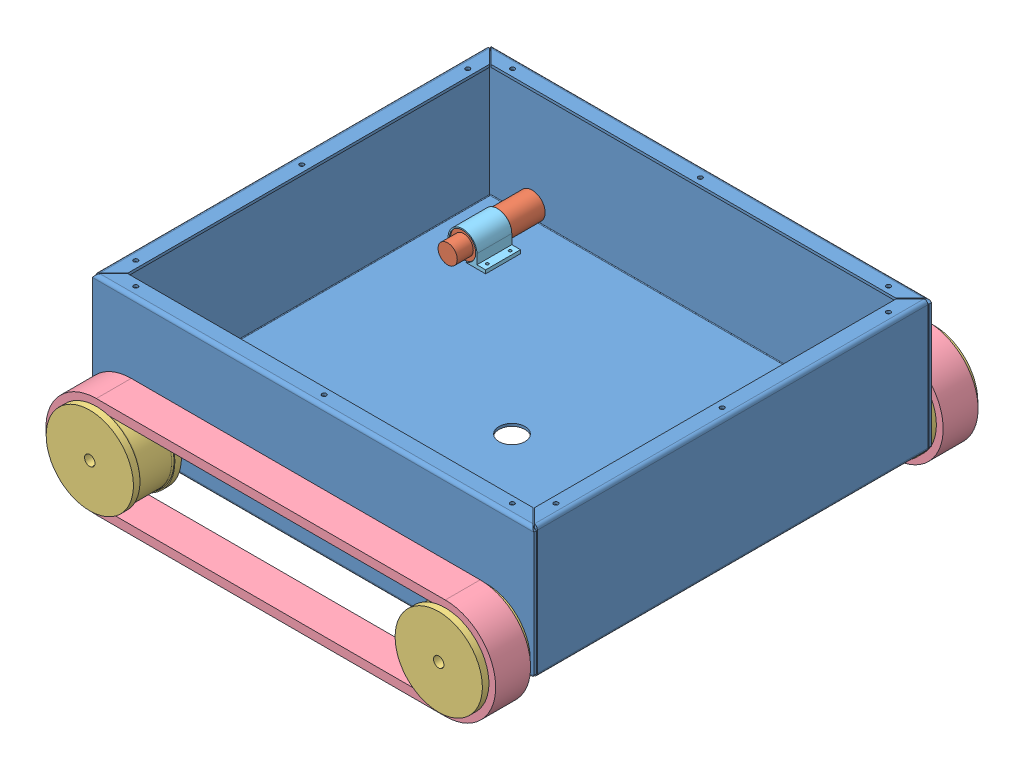
SolidWorks assembly assume4, configuration Default. Lengths in mm.
Overall size (594.52 201.03 568).
19 component instances, 8 part files, 19 mates.
Components (placement in the parent):
- body-1: body [Default] at (0 42.0634 0) size (506.34 150.02 456.02)
- dunker-motor-1: dunker-motor [Default] at (-200 57.8 184.6) size (30 30 138.75)
- dunker-motor-2: dunker-motor [Default] at (200 57.8 184.6) size (30 30 138.75)
- Rim1-1: Rim1 [Default] at (-218.7342 47.2529 252.8765) x (0 0 -1) z (-0.490584 0.871394 0) size (55 100 100)
- Rim1-2: Rim1 [Default] at (187.4918 75.2859 252.8765) x (0 0 -1) z (0.813332 0.5818 0) size (55 100 100)
- sair-1: sair [Default] at (-74.1917 57.8 236.5) x (1 0 0) z (0 -1 0) size (515.6 40 115.6)
- motor-holder-2: motor-holder [Default] at (-200 57.8 143.262) x (1 0 0) z (0 -1 0) size (53 40 31.6)
- motor-holder-3: motor-holder [Default] at (200 57.8 143.262) x (1 0 0) z (0 -1 0) size (53 40 31.6)
- motor-holder-4: motor-holder [Default] at (-200 57.8 -143.262) x (-1 0 0) z (0 -1 0) size (53 40 31.6)
- motor-holder-5: motor-holder [Default] at (200 57.8 -143.262) x (-1 0 0) z (0 -1 0) size (53 40 31.6)
- dunker-motor-3: dunker-motor [Default] at (-200 57.8 -184.6) x (-1 0 0) z (0 0 -1) size (30 30 138.75)
- dunker-motor-4: dunker-motor [Default] at (200 57.8 -184.6) x (-1 0 0) z (0 0 -1) size (30 30 138.75)
- Rim1-3: Rim1 [Default] at (-218.7342 47.2529 -252.8765) x (0 0 1) z (0.490584 -0.871394 0) size (55 100 100)
- Rim1-4: Rim1 [Default] at (187.4918 75.2859 -252.8765) x (0 0 1) z (-0.813332 -0.5818 0) size (55 100 100)
- sair-2: sair [Default] at (-74.1917 57.8 -236.5) x (1 0 0) z (0 1 0) size (515.6 40 115.6)
- cleaning part-1: cleaning part [Default] at (-305.4353 -118.1011 104.5044) x (1 0 0) z (0 1 0) size (115.57 320 56.98)
  - holder2-1: holder2 [Default] at (565.4382 75.7061 153.1645) size (72.07 200 12.5)
  - Part3-1: Part3 [Default] at (47.6736 218.1083 165.1645) x (-1 0 0) z (0 0 1) size (62 307 39.51)
  - brush 2-2: brush 2 [Default] at (24.6736 252.0044 137.1645) x (1 0 0) z (0 -1 0) size (52.04 51.98 320)
Mates (geometry in assembly coordinates):
- Coincident2: coincident aligned: plane of body-1 through (0 42.0634 0) normal (0 0 1)
- Coincident3: coincident aligned: plane of body-1 through (0 42.0634 0) normal (1 0 0)
- Concentric1: concentric anti-aligned: cylinder of body-1 through (200 57.8 -228.0075) axis (0 0 1) radius 3.25; cylinder of dunker-motor-2 through (200 57.8 265) axis (0 0 -1) radius 3
- Coincident4: coincident anti-aligned: plane of body-1 through (0 42.0634 225) normal (0 0 -1); plane of dunker-motor-2 through (200 57.8 225) normal (0 0 1)
- Concentric2: concentric anti-aligned: cylinder of body-1 through (-200 57.8 -228.0075) axis (0 0 1) radius 3.25; cylinder of dunker-motor-1 through (-200 57.8 265) axis (0 0 -1) radius 3
- Coincident5: coincident anti-aligned: plane of body-1 through (0 42.0634 225) normal (0 0 -1); plane of dunker-motor-1 through (-200 57.8 225) normal (0 0 1)
- Concentric3: concentric aligned: cylinder of dunker-motor-2 through (200 57.8 265) axis (0 0 -1) radius 3; cylinder of Rim1-2 through (200 57.8 284) axis (0 0 -1) radius 6
- Concentric4: concentric aligned: cylinder of dunker-motor-2 through (200 57.8 265) axis (0 0 -1) radius 3; cylinder of Rim1-2 through (200 57.8 284) axis (0 0 -1) radius 6
- Distance1: distance = 1 mm anti-aligned: plane of body-1 through (0 42.0634 228) normal (0 0 1); plane of Rim1-2 through (170.91 98.4666 229) normal (0 0 -1)
- Concentric5: concentric aligned: cylinder of dunker-motor-1 through (-200 57.8 265) axis (0 0 -1) radius 3; cylinder of Rim1-1 through (-200 57.8 284) axis (0 0 -1) radius 6
- Distance2: distance = 1 mm anti-aligned: plane of body-1 through (0 42.0634 228) normal (0 0 1); plane of Rim1-1 through (-243.5697 33.2708 229) normal (0 0 -1)
- Concentric7: concentric aligned: line of dunker-motor-1 through (-200 57.8 223) axis (0 0 -1); cylinder of sair-1 through (-200 57.8 276.5) axis (0 0 -1) radius 47.8
- Concentric8: concentric aligned: cylinder of Rim1-2 through (200 57.8 229) axis (0 0 -1) radius 47.8; cylinder of sair-1 through (200 57.8 276.5) axis (0 0 -1) radius 47.8
- Coincident11: coincident anti-aligned: plane of Rim1-1 through (-243.5697 33.2708 236.5) normal (0 0 1); plane of sair-1 through (-200 57.8 236.5) normal (0 0 -1)
- Concentric9: concentric anti-aligned: cylinder of dunker-motor-1 through (-200 57.8 144.6) axis (0 0 1) radius 15; cylinder of motor-holder-2 through (-200 57.8 183.262) axis (0 0 -1) radius 15.2
- Parallel2: parallel anti-aligned: plane of body-1 through (0 42.0634 0) normal (0 1 0); plane of motor-holder-2 through (-200 42.7 183.262) normal (0 -1 0)
- Coincident10: coincident anti-aligned: plane of sair-1 through (-200 0 276.5) normal (0 -1 0)
- Coincident12: coincident: plane of body-1 through (0 39.0634 0) normal (0 -1 0); plane of cleaning part-1/holder2-1 through (3.7529 39.0634 -72.9636) normal (0 1 0)
- Distance3: distance = 72 mm aligned: plane of cleaning part-1/Part3-1 through (-262.7617 47.0634 156) normal (0 0 1); plane of body-1 through (0 42.0634 228) normal (0 0 1)
